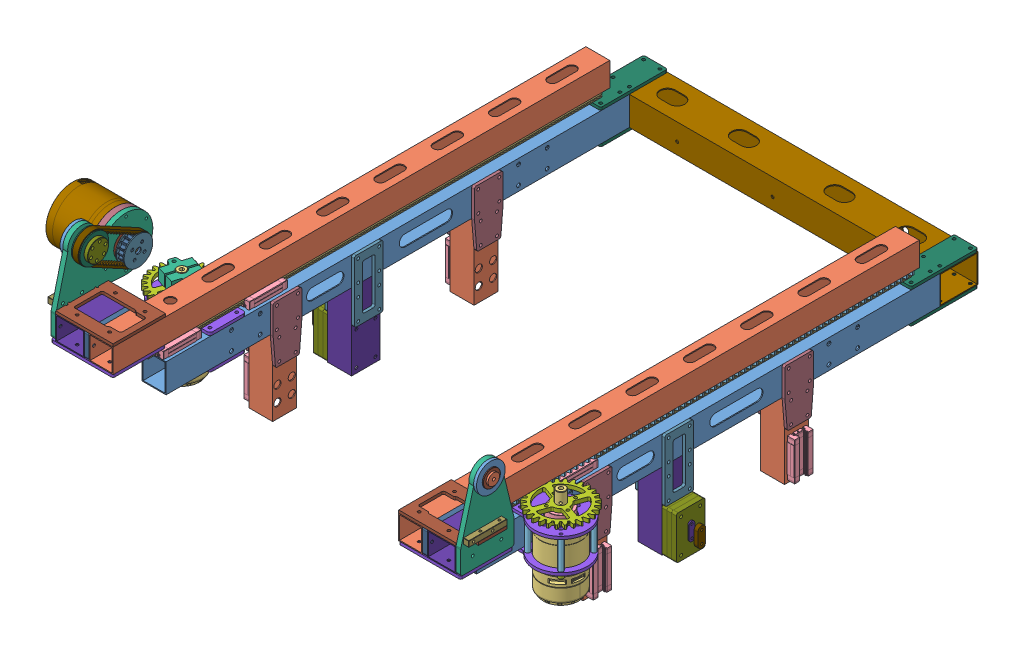
SolidWorks assembly 前探2.0, configuration 默认. Lengths in mm.
Overall size (521.63 224 581.5).
126 component instances, 37 part files, 323 mates.
Components (placement in the parent):
- 30x25x1铝方管-2: 30x25x1铝方管 [前探底管] at (162.5 0 0) size (25 30 485)
- 25x25x1铝方管-1: 25x25x1铝方管 [前探长管镜像] at (-162.5 43.5 38) size (25 25 520)
- 25x25x1铝方管-2: 25x25x1铝方管 [前探长管] at (162.5 43.5 39) size (25 25 520)
- RoboMaster M3508直流无刷减速电机-1: RoboMaster M3508直流无刷减速电机 [默认] at (-216.3113 -71.441 182.0369) x (0.14601 0 0.989283) z (0 1 0) size (42 42.01 98.4)
- 推力球轴承-1: 推力球轴承 [51100 10*24*9] at (-198.5 17 177.6) x (-0.941237 0 -0.337746) z (0.337746 0 -0.941237) size (24 9 24)
- 304不锈钢接线柱-1: 304不锈钢接线柱 [M3*30-5] at (-215.8241 0 160.2759) x (0.012605 0 0.999921) z (0 1 0) size (5 5 30)
- 304不锈钢接线柱-3: 304不锈钢接线柱 [M3*30-5] at (-215.8241 0 194.9241) x (-0.333238 0 0.942843) z (0 1 0) size (5 5 30)
- 304不锈钢接线柱-4: 304不锈钢接线柱 [M3*30-5] at (-181.1759 0 160.2759) x (-0.657276 0 0.75365) z (0 1 0) size (5 5 30)
- RoboMaster M3508直流无刷减速电机-2: RoboMaster M3508直流无刷减速电机 [默认] at (206.3813 -71.441 194.1776) x (0.940674 0 -0.339312) z (0 1 0) size (42 42.01 98.4)
- 推力球轴承-2: 推力球轴承 [51100 10*24*9] at (198.5 17 177.6) x (0.998455 0 0.055559) z (-0.055559 0 0.998455) size (24 9 24)
- 304不锈钢接线柱-5: 304不锈钢接线柱 [M3*30-5] at (215.8241 0 160.2759) x (-0.333238 0 0.942843) z (0 1 0) size (5 5 30)
- 304不锈钢接线柱-6: 304不锈钢接线柱 [M3*30-5] at (215.8241 0 194.9241) x (-0.485899 0 0.874015) z (0 1 0) size (5 5 30)
- 304不锈钢接线柱-7: 304不锈钢接线柱 [M3*30-5] at (181.1759 0 194.9241) x (-0.280607 0 0.959823) z (0 1 0) size (5 5 30)
- 304不锈钢接线柱-8: 304不锈钢接线柱 [M3*30-5] at (181.1759 0 160.2759) x (-0.117969 0 0.993017) z (0 1 0) size (5 5 30)
- 横移连接板-1: 横移连接板 [电机安装板] at (-210 43.5 263) x (0 0 1) z (-1 0 0) size (101.67 92 5)
- 12.9级圆柱头螺钉-2: 12.9级圆柱头螺钉 [M3*8] at (-215.8241 -21 194.9241) x (-0.034714 0 -0.999397) z (0 -1 0) size (5.68 5.68 11)
- 12.9级圆柱头螺钉-3: 12.9级圆柱头螺钉 [M3*8] at (-215.8241 -21 160.2759) x (-0.784933 0 -0.61958) z (0 -1 0) size (5.68 5.68 11)
- 12.9级圆柱头螺钉-4: 12.9级圆柱头螺钉 [M3*8] at (-181.1759 -21 160.2759) x (0.893078 0 -0.449902) z (0 -1 0) size (5.68 5.68 11)
- 12.9级圆柱头螺钉-5: 12.9级圆柱头螺钉 [M3*8] at (181.1759 -21 160.2759) x (0.99769 0 0.06793) z (0 -1 0) size (5.68 5.68 11)
- 12.9级圆柱头螺钉-6: 12.9级圆柱头螺钉 [M3*8] at (215.8241 -21 160.2759) x (0.98152 0 0.19136) z (0 -1 0) size (5.68 5.68 11)
- 12.9级圆柱头螺钉-7: 12.9级圆柱头螺钉 [M3*8] at (215.8241 -21 194.9241) x (0.999534 0 -0.03052) z (0 -1 0) size (5.68 5.68 11)
- 12.9级圆柱头螺钉-8: 12.9级圆柱头螺钉 [M3*8] at (181.1759 -21 194.9241) x (0.99867 0 -0.051563) z (0 -1 0) size (5.68 5.68 11)
- 12.9级圆柱头螺钉-9: 12.9级圆柱头螺钉 [M3*5] at (155 11 230.55) x (0.994595 0 0.103835) z (0 -1 0) size (5.68 5.68 8)
- 12.9级圆柱头螺钉-10: 12.9级圆柱头螺钉 [M3*5] at (170 11 230.55) x (0.998824 0 -0.048475) z (0 -1 0) size (5.68 5.68 8)
- 12.9级圆柱头螺钉-11: 12.9级圆柱头螺钉 [M3*5] at (170 11 214.55) x (0.998723 0 -0.050526) z (0 -1 0) size (5.68 5.68 8)
- 12.9级圆柱头螺钉-12: 12.9级圆柱头螺钉 [M3*5] at (155 11 214.55) x (0.998723 0 -0.050526) z (0 -1 0) size (5.68 5.68 8)
- 12.9级圆柱头螺钉-13: 12.9级圆柱头螺钉 [M3*5] at (170 11 140.65) x (-0.565957 0 0.824435) z (0 -1 0) size (5.68 5.68 8)
- 12.9级圆柱头螺钉-16: 12.9级圆柱头螺钉 [M3*5] at (155 11 140.65) x (0.977106 0 0.212755) z (0 -1 0) size (5.68 5.68 8)
- 12.9级圆柱头螺钉-17: 12.9级圆柱头螺钉 [M3*5] at (170 11 124.65) x (-0.206211 0 0.978508) z (0 -1 0) size (5.68 5.68 8)
- 12.9级圆柱头螺钉-18: 12.9级圆柱头螺钉 [M3*5] at (155 11 124.65) x (0.595095 0 -0.803655) z (0 -1 0) size (5.68 5.68 8)
- 12.9级圆柱头螺钉-19: 12.9级圆柱头螺钉 [M3*5] at (-155 11.0016 230.55) x (0.978167 0 0.207821) z (0 -1 0) size (5.68 5.68 8)
- 12.9级圆柱头螺钉-20: 12.9级圆柱头螺钉 [M3*5] at (-170 11 230.55) x (0.999805 0 0.019757) z (0 -1 0) size (5.68 5.68 8)
- 12.9级圆柱头螺钉-21: 12.9级圆柱头螺钉 [M3*5] at (-155 11.0163 214.55) x (0.980556 0 -0.196239) z (0 -1 0) size (5.68 5.68 8)
- 12.9级圆柱头螺钉-22: 12.9级圆柱头螺钉 [M3*5] at (-170 11 214.55) x (0.907226 0 -0.420643) z (0 -1 0) size (5.68 5.68 8)
- 12.9级圆柱头螺钉-23: 12.9级圆柱头螺钉 [M3*5] at (-155 11 140.65) x (0.937372 0 -0.348331) z (0 -1 0) size (5.68 5.68 8)
- 12.9级圆柱头螺钉-24: 12.9级圆柱头螺钉 [M3*5] at (-170 11 140.65) x (-0.229443 0 -0.973322) z (0 -1 0) size (5.68 5.68 8)
- 12.9级圆柱头螺钉-25: 12.9级圆柱头螺钉 [M3*5] at (-155 11 124.65) x (0.655383 0 -0.755297) z (0 -1 0) size (5.68 5.68 8)
- 12.9级圆柱头螺钉-26: 12.9级圆柱头螺钉 [M3*5] at (-170 11 124.65) x (-0.78488 0 -0.619648) z (0 -1 0) size (5.68 5.68 8)
- 横移连接板-2: 横移连接板 [转轴转点] at (215 43.5 263) x (0 0 1) z (-1 0 0) size (56 92 5)
- 支撑连接板-1: 支撑连接板 [右] at (182.5 28 271.5) x (1 0 0) z (0 1 0) size (65 55 3.23)
- 支撑连接板-2: 支撑连接板 [左] at (-182.5 28 270.5) x (1 0 0) z (0 1 0) size (341.52 580.5 35.52)
- 4310 减速电机 3D 20221104_defeature-1: 4310 减速电机 3D 20221104_defeature [默认] at (-259 83 224.3345) x (0 -0.927289 0.374346) z (0 0.374346 0.927289) size (56 46 56)
- 小带轮-1: 小带轮 [主动轮] at (-205.1 83 224.3345) x (1 0 0) z (0 -0.853122 0.521711) size (7 27.19 27.51)
- 法兰轴承-1: 法兰轴承 [17*26*5-1.1] at (-216.1 83 224.3345) x (0 -0.997676 0.068144) z (0 0.068144 0.997676) size (28 5 28)
- 4310传动法兰-1: 4310传动法兰 [默认] at (-220 83 224.3345) x (0 0.302939 -0.95301) z (1 0 0) size (33 33 19.9)
- 小带轮-2: 小带轮 [从动轮] at (-198.1 108 270.5) x (-1 0 0) z (0 -0.949657 -0.313291) size (7 27.19 27.51)
- 4310安装垫块-1: 4310安装垫块 [默认] at (-215 83 224.3345) x (0 0.536766 0.843731) z (-1 0 0) size (56 56 6)
- 同步带轮挡板-1: 同步带轮挡板 [默认] at (-206.1 83 224.3345) x (0 -0.521711 -0.853122) z (1 0 0) size (30 30 1)
- 同步带轮挡板-2: 同步带轮挡板 [默认] at (-197.1 83 224.3345) x (0 0.521711 0.853122) z (-1 0 0) size (30 30 1)
- 同步带轮挡板1-1: 同步带轮挡板1 [默认] at (-197.1 108 270.5) x (0 0.949657 0.313291) z (-1 0 0) size (30 30 1)
- 同步带轮挡板1-2: 同步带轮挡板1 [默认] at (-206.1 108 270.5) x (0 -0.203511 -0.979073) z (1 0 0) size (30 30 1)
- 横移转点法兰-1: 横移转点法兰 [默认] at (-193 108 270.5) x (0 0.949657 0.313291) z (-1 0 0) size (22 22 26.1)
- 25x30x1铝方管-1: 25x30x1铝方管 [前探管] at (-195 43.5 270.5) size (30 25 55)
- 25x30x1铝方管-2: 25x30x1铝方管 [前探管] at (195 43.5 271.5) size (30 25 55)
- 法兰轴承-2: 法兰轴承 [8*16*5-1.1] at (-208.9 108 270.5) x (0 -0.454379 0.890809) z (0 -0.890809 -0.454379) size (18 5 18)
- 法兰轴承-3: 法兰轴承 [8*16*5-1.1] at (208.9 108 270.5) x (0 -0.670714 0.741716) z (0 0.741716 0.670714) size (18 5 18)
- 同步带1-1: 同步带1 [默认] at (-201.6 108 270.5) x (1 0 0) z (0 0.47619 0.879342) size (6 30.99 83.49)
- 法兰轴承-4: 法兰轴承 [8*16*5-1.1] at (219.1 108 270.5) x (0 -0.846571 -0.532276) z (0 0.532276 -0.846571) size (18 5 18)
- 横移转点垫板-1: 横移转点垫板 [默认] at (215 108 270.5) x (0 -0.116472 -0.993194) z (1 0 0) size (30 30 3)
- 横移转点垫板-2: 横移转点垫板 [默认] at (-218 108 270.5) x (0 0.20708 -0.978324) z (1 0 0) size (30 30 3)
- 法兰轴承-5: 法兰轴承 [8*16*5-1.1] at (-219.1 108 270.5) x (0 -0.931071 0.364837) z (0 0.364837 0.931071) size (18 5 18)
- 转点垫片-1: 转点垫片 [默认] at (-219.1 108 270.5) x (0 0.356837 0.934167) z (-1 0 0) size (12 12 2)
- 转点垫片-2: 转点垫片 [默认] at (221.1 108 270.5) x (0 0.710644 0.703552) z (-1 0 0) size (12 12 2)
- 上银直线导轨线性滑轨MGN-C-O╱MGN-H-O[MGN9H2R475ZACI＋-O]_2-1: 上银直线导轨线性滑轨MGN-C-O╱MGN-H-O[MGN9H2R475ZACI＋-O]_2 [MGN9H-O] at (-162.5 22.8 15.5) x (-1 0 0) z (0 0 1) size (9 6.5 475)
- 上银直线导轨线性滑轨MGN-C-O╱MGN-H-O[MGN9H2R475ZACI＋-O]_1-1: 上银直线导轨线性滑轨MGN-C-O╱MGN-H-O[MGN9H2R475ZACI＋-O]_1 [MGN9H-O] at (-162.5 22.8 222.55) x (-1 0 0) z (0 0 1) size (20 7.8 39.98)
- 上银直线导轨线性滑轨MGN-C-O╱MGN-H-O[MGN9H2R475ZACI＋-O]_1-2: 上银直线导轨线性滑轨MGN-C-O╱MGN-H-O[MGN9H2R475ZACI＋-O]_1 [MGN9H-O] at (-162.5 22.8 132.65) x (-1 0 0) z (0 0 1) size (20 7.8 39.98)
- 30x25x1铝方管-6: 30x25x1铝方管 [前探底管] at (-162.5 0 0) size (25 30 485)
- 上银直线导轨线性滑轨MGN-C-O╱MGN-H-O[MGN9H2R475ZACI＋-O]_2-2: 上银直线导轨线性滑轨MGN-C-O╱MGN-H-O[MGN9H2R475ZACI＋-O]_2 [MGN9H-O] at (162.5 22.8 16.5) x (-1 0 0) z (0 0 1) size (9 6.5 475)
- 上银直线导轨线性滑轨MGN-C-O╱MGN-H-O[MGN9H2R475ZACI＋-O]_1-3: 上银直线导轨线性滑轨MGN-C-O╱MGN-H-O[MGN9H2R475ZACI＋-O]_1 [MGN9H-O] at (162.5 22.8 222.55) x (-1 0 0) z (0 0 1) size (20 7.8 39.98)
- 上银直线导轨线性滑轨MGN-C-O╱MGN-H-O[MGN9H2R475ZACI＋-O]_1-4: 上银直线导轨线性滑轨MGN-C-O╱MGN-H-O[MGN9H2R475ZACI＋-O]_1 [MGN9H-O] at (162.5 22.8 132.65) x (-1 0 0) z (0 0 1) size (20 7.8 39.98)
- 齿条2X76-1: 齿条2X76 [默认] at (168 31 244) x (0 0 -1) z (0 -1 0) size (465 14.5 6)
- 齿条2X76-3: 齿条2X76 [默认] at (-168 25 243) x (0 0 -1) z (0 1 0) size (465 14.5 6)
- 2孔夹紧联轴器-1: 2孔夹紧联轴器 [默认] at (-198.5 30 177.6) x (-0.289177 0 0.957276) z (0 1 0) size (28 32 12)
- 3508前探电机安装板-3: 3508前探电机安装板 [默认] at (-225 19 185.3862) x (0 0 1) z (0 -1 0) size (80 120 0)
- 圆柱齿轮28×2-1: 圆柱齿轮28×2 [默认] at (-198.5 30 177.6) x (0.942893 0 0.333096) z (0 -1 0) size (59.77 59.77 4)
- 前探3508安装板-1: 前探3508安装板 [3508安装板] at (-198.5 16.5 177.6) x (0 0 -1) z (0 1 0) size (55 76 3)
- 2孔夹紧联轴器-2: 2孔夹紧联轴器 [默认] at (198.5 30 177.6) x (-0.289177 0 0.957276) z (0 1 0) size (28 32 12) (hidden)
- 圆柱齿轮28×2-2: 圆柱齿轮28×2 [默认] at (198.5 30 177.6) x (0.942893 0 0.333096) z (0 -1 0) size (59.77 59.77 4)
- 前探3508安装板-2: 前探3508安装板 [3508安装板] at (198.5 16.5 177.6) x (0 0 -1) z (0 -1 0) size (55 76 3)
- 40x30x1铝方管-1: 40x30x1铝方管 [默认] at (0 0 -262.5) x (0 0 1) z (-1 0 0) size (40 30 350)
- 前探3508安装板-3: 前探3508安装板 [下端固定板] at (-198.5 -16.5 177.6) x (0 0 -1) z (0 1 0) size (55 76 3)
- 304不锈钢接线柱-9: 304不锈钢接线柱 [M3*30-5] at (-181.1759 0 194.9241) x (-0.000437 0 1) z (0 1 0) size (5 5 30)
- 12.9级圆柱头螺钉-27: 12.9级圆柱头螺钉 [M3*8] at (-181.1759 -21 194.9241) x (-0.034714 0 -0.999397) z (0 -1 0) size (5.68 5.68 11)
- 前探3508安装板-4: 前探3508安装板 [下端固定板] at (198.5 -16.5 177.6) x (0 0 -1) z (0 -1 0) size (55 76 3)
- 25x25x1铝方管-3: 25x25x1铝方管 [抬升滑块安装管] at (162.5 -55 118.4) x (1 0 0) z (0 -1 0) size (25 25 80)
- 25x25x1铝方管-4: 25x25x1铝方管 [抬升滑块安装管] at (162.5 -55 -92.4) x (1 0 0) z (0 -1 0) size (25 25 80)
- 上银直线导轨线性滑轨MGN-C-O╱MGN-H-O[MGN9H2R475ZACI＋-O]_1-5: 上银直线导轨线性滑轨MGN-C-O╱MGN-H-O[MGN9H2R475ZACI＋-O]_1 [MGN9H-O] at (182.8 -72.05 118.4) x (0 0 -1) z (0 1 0) size (20 7.8 39.98)
- 上银直线导轨线性滑轨MGN-C-O╱MGN-H-O[MGN9H2R475ZACI＋-O]_1-6: 上银直线导轨线性滑轨MGN-C-O╱MGN-H-O[MGN9H2R475ZACI＋-O]_1 [MGN9H-O] at (182.8 -72.05 -92.4) x (0 0 -1) z (0 1 0) size (20 7.8 39.98)
- 25x25x1铝方管-5: 25x25x1铝方管 [抬升滑块安装管] at (-162.5 -55 118.4) x (-1 0 0) z (0 -1 0) size (25 25 80)
- 25x25x1铝方管-6: 25x25x1铝方管 [抬升滑块安装管] at (-162.5 -55 -92.4) x (-1 0 0) z (0 -1 0) size (25 25 80)
- 上银直线导轨线性滑轨MGN-C-O╱MGN-H-O[MGN9H2R475ZACI＋-O]_1-7: 上银直线导轨线性滑轨MGN-C-O╱MGN-H-O[MGN9H2R475ZACI＋-O]_1 [MGN9H-O] at (-182.8 -72.05 -92.4) x (0 0 -1) z (0 -1 0) size (20 7.8 39.98)
- 上银直线导轨线性滑轨MGN-C-O╱MGN-H-O[MGN9H2R475ZACI＋-O]_1-8: 上银直线导轨线性滑轨MGN-C-O╱MGN-H-O[MGN9H2R475ZACI＋-O]_1 [MGN9H-O] at (-182.8 -72.05 118.4) x (0 0 -1) z (0 -1 0) size (20 7.8 39.98)
- 前探垫块-1: 前探垫块 [默认] at (-180 43.5 270.5) x (0 0 -1) z (1 0 0) size (55 25 5)
- 前探垫块-2: 前探垫块 [默认] at (175 43.5 271.5) x (0 0 -1) z (1 0 0) size (55 25 5)
- 前探加固板-1: 前探加固板 [默认] at (-180 59 270.5) x (0 0 1) z (0 -1 0) size (55 71 3)
- 四孔直角转接件-1: 四孔直角转接件 [上交角件] at (-218 62 275.5) x (0 1 0) z (0 0 1) size (6 6 40)
- 前探加固板-2: 前探加固板 [默认] at (180 56 271.5) x (0 0 1) z (0 1 0) size (55 71 3)
- 四孔直角转接件-2: 四孔直角转接件 [上交角件] at (218 62 276.5) x (0 1 0) z (0 0 1) size (6 6 40)
- 25x30x1铝方管-3: 25x30x1铝方管 [抬升管] at (-162.5 -55 33.295) x (0 0 1) z (0 1 0) size (30 25 80)
- 25x30x1铝方管-4: 25x30x1铝方管 [抬升管] at (162.5 -55 33.295) x (0 0 -1) z (0 1 0) size (30 25 80)
- 抬升连接板1-1: 抬升连接板1 [默认] at (-176.5 0 -92.4) x (0 0 1) z (-1 0 0) size (30 60 3)
- 抬升连接板1-2: 抬升连接板1 [默认] at (-176.5 0 118.4) x (0 0 -1) z (1 0 0) size (30 60 3)
- 抬升连接板1-3: 抬升连接板1 [默认] at (-148.5 0 -92.4) x (0 0 1) z (-1 0 0) size (30 60 3)
- 抬升连接板1-4: 抬升连接板1 [默认] at (-148.5 0 118.4) x (0 0 -1) z (1 0 0) size (30 60 3)
- 抬升连接板2-1: 抬升连接板2 [默认] at (-175 -17.5 33.295) x (0 0 1) z (-1 0 0) size (30 65 3)
- 抬升连接板2-2: 抬升连接板2 [默认] at (-147 -17.5 33.295) x (0 0 1) z (-1 0 0) size (30 65 3)
- 抬升连接板1-5: 抬升连接板1 [默认] at (176.5 0 118.4) x (0 0 -1) z (1 0 0) size (30 60 3)
- 抬升连接板1-6: 抬升连接板1 [默认] at (148.5 0 118.4) x (0 0 -1) z (1 0 0) size (30 60 3)
- 抬升连接板1-7: 抬升连接板1 [默认] at (176.5 0 -92.4) x (0 0 -1) z (1 0 0) size (30 60 3)
- 抬升连接板1-8: 抬升连接板1 [默认] at (148.5 0 -92.4) x (0 0 -1) z (1 0 0) size (30 60 3)
- 抬升连接板2-3: 抬升连接板2 [默认] at (178 -17.5 33.295) x (0 0 1) z (-1 0 0) size (30 65 3)
- 抬升连接板2-4: 抬升连接板2 [默认] at (150 -17.5 33.295) x (0 0 1) z (-1 0 0) size (30 65 3)
- 前探连接板-1: 前探连接板 [默认] at (-162.5 15 -247.5) x (0 0 -1) z (0 1 0) size (70 25 3)
- 前探连接板-2: 前探连接板 [默认] at (162.5 15 -247.5) x (0 0 -1) z (0 1 0) size (70 25 3)
- 前探连接板-3: 前探连接板 [默认] at (162.5 -18 -247.5) x (0 0 -1) z (0 1 0) size (70 25 3)
- 前探连接板-4: 前探连接板 [默认] at (-162.5 -18 -247.5) x (0 0 -1) z (0 1 0) size (70 25 3)
- 抬升链条连接-1: 抬升链条连接 [底层] at (-175 -72.5 33.295) x (0 0 1) z (-1 0 0) size (30 45 5)
- 抬升链条连接-2: 抬升链条连接 [二层] at (-180 -72.5 33.295) x (0 0 1) z (-1 0 0) size (30 45 5)
- 抬升链条连接-5: 抬升链条连接 [连接一层] at (-185 -72.5 33.295) x (0 0 1) z (-1 0 0) size (30 45 5)
- 链条连接垫块-1: 链条连接垫块 [默认] at (-190 -72.5 33.295) x (0 0 1) z (-1 0 0) size (6 18.7 1.31)
- 链条连接-1: 链条连接 [默认] at (-197.69 -72.5 33.295) x (0 0 1) z (-1 0 0) size (8 20.7 4)
- 抬升链条连接-6: 抬升链条连接 [底层] at (180 -72.5 33.295) x (0 0 1) z (-1 0 0) size (30 45 5)
- 抬升链条连接-8: 抬升链条连接 [底层] at (185 -72.5 33.295) x (0 0 1) z (-1 0 0) size (30 45 5)
- 抬升链条连接-9: 抬升链条连接 [连接一层] at (190 -72.5 33.295) x (0 0 1) z (-1 0 0) size (30 45 5)
- 链条连接垫块-2: 链条连接垫块 [默认] at (191.31 -72.5 33.295) x (0 0 1) z (-1 0 0) size (6 18.7 1.31)
- 链条连接-2: 链条连接 [默认] at (201.69 -72.5 33.295) x (0 0 1) z (-1 0 0) size (8 20.7 4)
Mates (geometry in assembly coordinates):
- 重合3: coincident aligned: plane of 30x25x1铝方管-2 through (162.5 0 0) normal (0 0 1)
- 重合4: coincident aligned: plane of 30x25x1铝方管-2 through (162.5 0 0) normal (0 1 0)
- 同心2: concentric anti-aligned: cylinder of RoboMaster M3508直流无刷减速电机-1 through (-198.5 42.3 177.6) axis (0 1 0) radius 5; cylinder of 推力球轴承-1 through (-198.5 26 177.6) axis (0 -1 0) radius 12
- 重合23: coincident anti-aligned: plane of RoboMaster M3508直流无刷减速电机-1 through (-209.1562 17 174.8713) normal (0 1 0); plane of 推力球轴承-1 through (-198.5 17 177.6) normal (0 -1 0)
- 同心19: concentric anti-aligned: cylinder of RoboMaster M3508直流无刷减速电机-2 through (198.5 42.3 177.6) axis (0 1 0) radius 5; cylinder of 推力球轴承-2 through (198.5 26 177.6) axis (0 -1 0) radius 5
- 重合44: coincident anti-aligned: plane of RoboMaster M3508直流无刷减速电机-2 through (197.9389 17 188.5857) normal (0 1 0); plane of 推力球轴承-2 through (198.5 17 177.6) normal (0 -1 0)
- 重合54: coincident aligned: plane of 25x25x1铝方管-1 through (-175 31 298) normal (0 -1 0); plane of 横移连接板-1 through (-215 31 243) normal (0 -1 0)
- 重合68: coincident anti-aligned: plane of 30x25x1铝方管-2 through (151 14 242.5) normal (0 -1 0); plane of 12.9级圆柱头螺钉-9 through (154.7051 14 233.3746) normal (0 1 0)
- 重合691: coincident anti-aligned: plane of 30x25x1铝方管-2 through (151 14 242.5) normal (0 -1 0); plane of 12.9级圆柱头螺钉-10 through (170.1377 14 233.3867) normal (0 1 0)
- 重合701: coincident anti-aligned: plane of 30x25x1铝方管-2 through (151 14 242.5) normal (0 -1 0); plane of 12.9级圆柱头螺钉-11 through (170.1435 14 217.3864) normal (0 1 0)
- 重合711: coincident anti-aligned: plane of 30x25x1铝方管-2 through (151 14 242.5) normal (0 -1 0); plane of 12.9级圆柱头螺钉-12 through (155.1435 14 217.3864) normal (0 1 0)
- 重合72: coincident anti-aligned: plane of 30x25x1铝方管-2 through (151 14 242.5) normal (0 -1 0); plane of 12.9级圆柱头螺钉-13 through (167.6586 14 139.0427) normal (0 1 0)
- 重合761: coincident anti-aligned: plane of 30x25x1铝方管-2 through (151 14 242.5) normal (0 -1 0); plane of 12.9级圆柱头螺钉-16 through (154.3958 14 143.425) normal (0 1 0)
- 重合77: coincident anti-aligned: plane of 30x25x1铝方管-2 through (151 14 242.5) normal (0 -1 0); plane of 12.9级圆柱头螺钉-17 through (167.221 14 124.0644) normal (0 1 0)
- 重合78: coincident anti-aligned: plane of 30x25x1铝方管-2 through (151 14 242.5) normal (0 -1 0); plane of 12.9级圆柱头螺钉-18 through (157.2824 14 126.3401) normal (0 1 0)
- 平行8: parallel aligned: plane of 25x25x1铝方管-2 through (150 31 299) normal (0 -1 0); plane of 横移连接板-2 through (210 31 243) normal (0 -1 0)
- 同心427: concentric aligned: cylinder of 横移连接板-1 through (-224 108 270.5) axis (1 0 0) radius 8; cylinder of 横移连接板-2 through (201 108 270.5) axis (1 0 0) radius 8
- 重合786: coincident anti-aligned: plane of 25x25x1铝方管-2 through (150 31 299) normal (0 -1 0); plane of 支撑连接板-1 through (182.5 31 271.5) normal (0 1 0)
- 重合787: coincident aligned: plane of 25x25x1铝方管-2 through (150 31 299) normal (-1 0 0); plane of 支撑连接板-1 through (150 31 299) normal (-1 0 0)
- 重合788: coincident aligned: plane of 25x25x1铝方管-2 through (162.5 43.5 299) normal (0 0 1); plane of 支撑连接板-1 through (150 31 299) normal (0 0 1)
- 重合789: coincident anti-aligned: plane of 25x25x1铝方管-1 through (-175 31 298) normal (0 -1 0); plane of 支撑连接板-2 through (-182.5 31 270.5) normal (0 1 0)
- 重合790: coincident aligned: plane of 25x25x1铝方管-1 through (-150 31 298) normal (1 0 0); plane of 支撑连接板-2 through (-150 31 298) normal (1 0 0)
- 重合791: coincident aligned: plane of 25x25x1铝方管-1 through (-162.5 43.5 298) normal (0 0 1); plane of 支撑连接板-2 through (-215 31 298) normal (0 0 1)
- 重合792: coincident aligned: plane of 25x25x1铝方管-1 through (-162.5 43.5 298) normal (0 0 1); plane of 横移连接板-1 through (-301.6256 31 298) normal (0 0 1)
- 同心428: concentric anti-aligned: cylinder of 横移连接板-1 through (-220 83 224.3345) axis (1 0 0) radius 13; cylinder of 法兰轴承-1 through (-211.1 83 224.3345) axis (-1 0 0) radius 13
- 重合793: coincident anti-aligned: plane of 横移连接板-1 through (-215 43.5 263) normal (-1 0 0); plane of 法兰轴承-1 through (-215 83 224.3345) normal (1 0 0)
- 同心429: concentric aligned: cylinder of 4310 减速电机 3D 20221104_defeature-1 through (-259 83 224.3345) axis (-1 0 0) radius 28; cylinder of 法兰轴承-1 through (-211.1 83 224.3345) axis (-1 0 0) radius 8.5
- 距离15: distance = 6 mm anti-aligned: plane of 4310 减速电机 3D 20221104_defeature-1 through (-221 63.0633 232.383) normal (1 0 0); plane of 横移连接板-1 through (-215 43.5 263) normal (-1 0 0)
- 同心430: concentric aligned: cylinder of 法兰轴承-1 through (-211.1 83 224.3345) axis (-1 0 0) radius 8.5; cylinder of 4310传动法兰-1 through (-206.1 83 224.3345) axis (-1 0 0) radius 8.5
- 重合794: coincident anti-aligned: plane of 4310 减速电机 3D 20221104_defeature-1 through (-220 84.7781 228.7392) normal (1 0 0); plane of 4310传动法兰-1 through (-220 83 224.3345) normal (-1 0 0)
- 同心431: concentric anti-aligned: cylinder of 小带轮-1 through (-208.1 83 224.3345) axis (1 0 0) radius 3; cylinder of 4310传动法兰-1 through (-206.1 83 224.3345) axis (-1 0 0) radius 8.5
- 同心432: concentric anti-aligned: cylinder of 横移连接板-1 through (-224 108 270.5) axis (1 0 0) radius 8; cylinder of 小带轮-2 through (-195.1 108 270.5) axis (-1 0 0) radius 5
- 同心433: concentric aligned: cylinder of 4310 减速电机 3D 20221104_defeature-1 through (-221 83 224.3345) axis (1 0 0) radius 28; cylinder of 4310安装垫块-1 through (-221 83 224.3345) axis (1 0 0) radius 28
- 重合796: coincident anti-aligned: plane of 横移连接板-1 through (-215 43.5 263) normal (-1 0 0); plane of 4310安装垫块-1 through (-215 83 224.3345) normal (1 0 0)
- 同心434: concentric anti-aligned: cylinder of 4310传动法兰-1 through (-200.1 83 224.3345) axis (-1 0 0) radius 3; cylinder of 同步带轮挡板-1 through (-206.1 83 224.3345) axis (1 0 0) radius 3
- 重合797: coincident anti-aligned: plane of 4310传动法兰-1 through (-206.1 83 224.3345) normal (1 0 0); plane of 同步带轮挡板-1 through (-206.1 83 224.3345) normal (-1 0 0)
- 重合798: coincident anti-aligned: plane of 小带轮-1 through (-205.1 84.435 226.6811) normal (-1 0 0); plane of 同步带轮挡板-1 through (-205.1 83 224.3345) normal (1 0 0)
- 同心435: concentric anti-aligned: cylinder of 小带轮-1 through (-244.1 86.9128 230.733) axis (1 0 0) radius 1.525; cylinder of 同步带轮挡板-1 through (-205.1 86.9128 230.733) axis (-1 0 0) radius 1.525
- 重合800: coincident anti-aligned: plane of 小带轮-1 through (-198.1 84.435 226.6811) normal (1 0 0); plane of 同步带轮挡板-2 through (-198.1 83 224.3345) normal (-1 0 0)
- 同心436: concentric anti-aligned: cylinder of 小带轮-1 through (-208.1 83 224.3345) axis (1 0 0) radius 3; cylinder of 同步带轮挡板-2 through (-197.1 83 224.3345) axis (-1 0 0) radius 3
- 同心437: concentric aligned: cylinder of 小带轮-1 through (-244.1 86.9128 230.733) axis (1 0 0) radius 1.525; cylinder of 同步带轮挡板-2 through (-198.1 86.9128 230.733) axis (1 0 0) radius 1.525
- 重合801: coincident aligned: plane of 小带轮-1 through (-198.1 84.435 226.6811) normal (1 0 0); plane of 小带轮-2 through (-198.1 108.8617 267.8879) normal (1 0 0)
- 重合802: coincident anti-aligned: plane of 小带轮-2 through (-198.1 108.8617 267.8879) normal (1 0 0); plane of 同步带轮挡板1-1 through (-198.1 108 270.5) normal (-1 0 0)
- 同心438: concentric anti-aligned: cylinder of 小带轮-2 through (-173.1 115.8326 268.8719) axis (-1 0 0) radius 1.5; cylinder of 同步带轮挡板1-1 through (-198.1 115.8326 268.8719) axis (1 0 0) radius 1.5
- 同心439: concentric anti-aligned: cylinder of 小带轮-2 through (-195.1 108 270.5) axis (-1 0 0) radius 5; cylinder of 同步带轮挡板1-1 through (-198.1 108 270.5) axis (1 0 0) radius 5
- 重合8031: coincident anti-aligned: plane of 小带轮-2 through (-205.1 108.8617 267.8879) normal (-1 0 0); plane of 同步带轮挡板1-2 through (-205.1 108 270.5) normal (1 0 0)
- 同心440: concentric aligned: cylinder of 小带轮-2 through (-195.1 108 270.5) axis (-1 0 0) radius 5; cylinder of 同步带轮挡板1-2 through (-205.1 108 270.5) axis (-1 0 0) radius 5
- 同心441: concentric anti-aligned: cylinder of 同步带轮挡板1-1 through (-198.1 113.3263 276.4692) axis (1 0 0) radius 1.5; cylinder of 同步带轮挡板1-2 through (-205.1 113.3263 276.4692) axis (-1 0 0) radius 1.5
- 同心442: concentric anti-aligned: cylinder of 小带轮-2 through (-195.1 108 270.5) axis (-1 0 0) radius 5; cylinder of 横移转点法兰-1 through (-219.1 108 270.5) axis (1 0 0) radius 5
- 重合804: coincident anti-aligned: plane of 同步带轮挡板1-1 through (-197.1 108 270.5) normal (1 0 0); plane of 横移转点法兰-1 through (-197.1 108 270.5) normal (-1 0 0)
- 同心443: concentric aligned: cylinder of 同步带轮挡板1-1 through (-198.1 113.3263 276.4692) axis (1 0 0) radius 1.5; cylinder of 横移转点法兰-1 through (-197.1 113.3263 276.4692) axis (1 0 0) radius 1.5
- 重合806: coincident aligned: plane of 25x25x1铝方管-1 through (-162.5 43.5 298) normal (0 0 1); plane of 25x30x1铝方管-1 through (-195 43.5 298) normal (0 0 1)
- 重合807: coincident anti-aligned: plane of 支撑连接板-2 through (-182.5 31 270.5) normal (0 1 0); plane of 25x30x1铝方管-1 through (-210 31 298) normal (0 -1 0)
- 重合808: coincident anti-aligned: plane of 横移连接板-1 through (-210 43.5 263) normal (1 0 0); plane of 25x30x1铝方管-1 through (-210 31 298) normal (-1 0 0)
- 重合810: coincident aligned: plane of 支撑连接板-1 through (150 31 299) normal (0 0 1); plane of 25x30x1铝方管-2 through (195 43.5 299) normal (0 0 1)
- 重合811: coincident anti-aligned: plane of 支撑连接板-1 through (182.5 31 271.5) normal (0 1 0); plane of 25x30x1铝方管-2 through (180 31 299) normal (0 -1 0)
- 重合812: coincident anti-aligned: plane of 横移连接板-2 through (210 43.5 263) normal (-1 0 0); plane of 25x30x1铝方管-2 through (210 31 299) normal (1 0 0)
- 同心444: concentric aligned: cylinder of 横移连接板-1 through (-224 108 270.5) axis (1 0 0) radius 8; cylinder of 法兰轴承-2 through (-213.9 108 270.5) axis (1 0 0) radius 8
- 重合815: coincident anti-aligned: plane of 横移连接板-1 through (-210 43.5 263) normal (1 0 0); plane of 法兰轴承-2 through (-210 108 270.5) normal (-1 0 0)
- 同心445: concentric anti-aligned: cylinder of 横移连接板-2 through (201 108 270.5) axis (1 0 0) radius 8; cylinder of 法兰轴承-3 through (213.9 108 270.5) axis (-1 0 0) radius 8
- 重合816: coincident anti-aligned: plane of 横移连接板-2 through (210 43.5 263) normal (-1 0 0); plane of 法兰轴承-3 through (210 108 270.5) normal (1 0 0)
- 同心446: concentric aligned: cylinder of 同步带轮挡板-2 through (-198.1 83 224.3345) axis (1 0 0) radius 15; cylinder of 同步带1-1 through (-201.6 83 224.3345) axis (1 0 0) radius 15.493
- 同心447: concentric anti-aligned: cylinder of 同步带轮挡板1-1 through (-198.1 108 270.5) axis (1 0 0) radius 15; cylinder of 同步带1-1 through (-201.6 108 270.5) axis (-1 0 0) radius 15.493
- 宽度13: width anti-aligned: plane of 同步带1-1 through (-204.6 97.7179 276.0681) normal (-1 0 0); plane of 同步带1-1 through (-198.6 94.3764 277.8776) normal (1 0 0); plane of 同步带轮挡板-1 through (-205.1 83 224.3345) normal (1 0 0); plane of 同步带轮挡板-2 through (-198.1 83 224.3345) normal (-1 0 0)
- 同心448: concentric anti-aligned: cylinder of 法兰轴承-3 through (213.9 108 270.5) axis (-1 0 0) radius 4; cylinder of 法兰轴承-4 through (214.1 108 270.5) axis (1 0 0) radius 4
- 距离16: distance = 0.2 mm anti-aligned: plane of 法兰轴承-3 through (213.9 108 270.5) normal (1 0 0); plane of 法兰轴承-4 through (214.1 108 270.5) normal (-1 0 0)
- 同心449: concentric anti-aligned: cylinder of 法兰轴承-4 through (214.1 108 270.5) axis (1 0 0) radius 4; cylinder of 横移转点垫板-1 through (218 108 270.5) axis (-1 0 0) radius 8
- 重合8032: coincident anti-aligned: plane of 横移连接板-2 through (215 43.5 263) normal (1 0 0); plane of 横移转点垫板-1 through (215 108 270.5) normal (-1 0 0)
- 同心450: concentric anti-aligned: cylinder of 横移连接板-1 through (-257.4264 108 270.5) axis (1 0 0) radius 15; cylinder of 横移转点垫板-2 through (-215 108 270.5) axis (-1 0 0) radius 15
- 重合8033: coincident anti-aligned: plane of 横移连接板-1 through (-215 43.5 263) normal (-1 0 0); plane of 横移转点垫板-2 through (-215 108 270.5) normal (1 0 0)
- 同心451: concentric aligned: cylinder of 横移转点垫板-2 through (-215 108 270.5) axis (-1 0 0) radius 8; cylinder of 法兰轴承-5 through (-214.1 108 270.5) axis (-1 0 0) radius 8
- 重合8034: coincident anti-aligned: plane of 横移转点垫板-2 through (-218 108 270.5) normal (-1 0 0); plane of 法兰轴承-5 through (-218 108 270.5) normal (1 0 0)
- 同心452: concentric anti-aligned: cylinder of 横移转点法兰-1 through (-219.1 108 270.5) axis (-1 0 0) radius 1.25; cylinder of 转点垫片-1 through (-221.1 108 270.5) axis (1 0 0) radius 1.55
- 重合8035: coincident anti-aligned: plane of 法兰轴承-5 through (-219.1 108 270.5) normal (-1 0 0); plane of 转点垫片-1 through (-219.1 108 270.5) normal (1 0 0)
- 同心453: concentric anti-aligned: cylinder of 法兰轴承-3 through (213.9 108 270.5) axis (-1 0 0) radius 4; cylinder of 转点垫片-2 through (219.1 108 270.5) axis (1 0 0) radius 1.55
- 重合8036: coincident anti-aligned: plane of 法兰轴承-4 through (219.1 108 270.5) normal (1 0 0); plane of 转点垫片-2 through (219.1 108 270.5) normal (-1 0 0)
- 宽度14: width aligned: plane of 25x25x1铝方管-1 through (-150 31 298) normal (1 0 0); plane of 上银直线导轨线性滑轨MGN-C-O╱MGN-H-O[MGN9H2R475ZACI＋-O]_2-1 through (-175 31 298) normal (-1 0 0); plane of 25x25x1铝方管-1 through (-158 24.6775 253) normal (1 0 0); plane of 上银直线导轨线性滑轨MGN-C-O╱MGN-H-O[MGN9H2R475ZACI＋-O]_2-1 through (-167 24.6775 253) normal (-1 0 0)
- 重合8044: coincident anti-aligned: plane of 上银直线导轨线性滑轨MGN-C-O╱MGN-H-O[MGN9H2R475ZACI＋-O]_2-1 through (-166.6775 18.5 253) normal (0 -1 0); plane of 上银直线导轨线性滑轨MGN-C-O╱MGN-H-O[MGN9H2R475ZACI＋-O]_1-1 through (-166.6775 18.5 203.925) normal (0 1 0)
- 宽度15: width anti-aligned: plane of 上银直线导轨线性滑轨MGN-C-O╱MGN-H-O[MGN9H2R475ZACI＋-O]_1-1 through (-167 24.6775 203.925) normal (1 0 0); plane of 上银直线导轨线性滑轨MGN-C-O╱MGN-H-O[MGN9H2R475ZACI＋-O]_2-1 through (-158 24.6775 203.925) normal (-1 0 0); plane of 上银直线导轨线性滑轨MGN-C-O╱MGN-H-O[MGN9H2R475ZACI＋-O]_1-1 through (-167 24.6775 253) normal (-1 0 0); plane of 上银直线导轨线性滑轨MGN-C-O╱MGN-H-O[MGN9H2R475ZACI＋-O]_2-1 through (-158 24.6775 253) normal (1 0 0)
- 宽度18: width anti-aligned: plane of 上银直线导轨线性滑轨MGN-C-O╱MGN-H-O[MGN9H2R475ZACI＋-O]_1-2 through (-172.5 17 147.3) normal (-1 0 0); plane of 上银直线导轨线性滑轨MGN-C-O╱MGN-H-O[MGN9H2R475ZACI＋-O]_2-1 through (-152.5 17 147.3) normal (1 0 0); plane of 上银直线导轨线性滑轨MGN-C-O╱MGN-H-O[MGN9H2R475ZACI＋-O]_1-2 through (-158 24.6775 253) normal (1 0 0); plane of 上银直线导轨线性滑轨MGN-C-O╱MGN-H-O[MGN9H2R475ZACI＋-O]_2-1 through (-167 24.6775 253) normal (-1 0 0)
- 距离18: distance = 50 mm anti-aligned: plane of 上银直线导轨线性滑轨MGN-C-O╱MGN-H-O[MGN9H2R475ZACI＋-O]_1-2 through (-162.5 32.2555 152.6) normal (0 0 1); plane of 上银直线导轨线性滑轨MGN-C-O╱MGN-H-O[MGN9H2R475ZACI＋-O]_1-1 through (-162.5 32.2555 202.6) normal (0 0 -1)
- 同心459: concentric anti-aligned: cylinder of 12.9级圆柱头螺钉-22 through (-170 19 214.55) axis (0 1 0) radius 1.5; cylinder of 上银直线导轨线性滑轨MGN-C-O╱MGN-H-O[MGN9H2R475ZACI＋-O]_1-1 through (-170 15 214.55) axis (0 -1 0) radius 1.5
- 同心460: concentric anti-aligned: cylinder of 12.9级圆柱头螺钉-25 through (-155 19 124.65) axis (0 1 0) radius 1.5; cylinder of 上银直线导轨线性滑轨MGN-C-O╱MGN-H-O[MGN9H2R475ZACI＋-O]_1-2 through (-155 15 124.65) axis (0 -1 0) radius 1.5
- 同心461: concentric anti-aligned: cylinder of 12.9级圆柱头螺钉-26 through (-170 19 124.65) axis (0 1 0) radius 1.5; cylinder of 上银直线导轨线性滑轨MGN-C-O╱MGN-H-O[MGN9H2R475ZACI＋-O]_1-2 through (-170 15 124.65) axis (0 -1 0) radius 1.5
- 同心462: concentric anti-aligned: cylinder of 12.9级圆柱头螺钉-24 through (-170 19 140.65) axis (0 1 0) radius 1.5; cylinder of 上银直线导轨线性滑轨MGN-C-O╱MGN-H-O[MGN9H2R475ZACI＋-O]_1-2 through (-170 15 140.65) axis (0 -1 0) radius 1.5
- 同心463: concentric anti-aligned: cylinder of 12.9级圆柱头螺钉-23 through (-155 19 140.65) axis (0 1 0) radius 1.5; cylinder of 上银直线导轨线性滑轨MGN-C-O╱MGN-H-O[MGN9H2R475ZACI＋-O]_1-2 through (-155 15 140.65) axis (0 -1 0) radius 1.5
- 同心464: concentric anti-aligned: cylinder of 12.9级圆柱头螺钉-19 through (-155 19.0016 230.55) axis (0 1 0) radius 1.5; cylinder of 上银直线导轨线性滑轨MGN-C-O╱MGN-H-O[MGN9H2R475ZACI＋-O]_1-1 through (-155 15 230.55) axis (0 -1 0) radius 1.5
- 同心465: concentric anti-aligned: cylinder of 12.9级圆柱头螺钉-21 through (-155 19.0163 214.55) axis (0 1 0) radius 1.5; cylinder of 上银直线导轨线性滑轨MGN-C-O╱MGN-H-O[MGN9H2R475ZACI＋-O]_1-1 through (-155 15 214.55) axis (0 -1 0) radius 1.5
- 同心466: concentric anti-aligned: cylinder of 12.9级圆柱头螺钉-20 through (-170 19 230.55) axis (0 1 0) radius 1.5; cylinder of 上银直线导轨线性滑轨MGN-C-O╱MGN-H-O[MGN9H2R475ZACI＋-O]_1-1 through (-170 15 230.55) axis (0 -1 0) radius 1.5
- 同心467: concentric anti-aligned: cylinder of 12.9级圆柱头螺钉-22 through (-170 19 214.55) axis (0 1 0) radius 1.5; cylinder of 上银直线导轨线性滑轨MGN-C-O╱MGN-H-O[MGN9H2R475ZACI＋-O]_1-1 through (-170 15 214.55) axis (0 -1 0) radius 1.5
- 对称1: symmetric aligned: plane of 30x25x1铝方管-2 through (150 -15 242.5) normal (-1 0 0); plane of 30x25x1铝方管-6 through (-150 -15 242.5) normal (1 0 0)
- 重合8050: coincident aligned: plane of 30x25x1铝方管-2 through (150 -15 242.5) normal (0 -1 0); plane of 30x25x1铝方管-6 through (-175 -15 242.5) normal (0 -1 0)
- 重合8051: coincident aligned: plane of 30x25x1铝方管-2 through (162.5 0 0) normal (0 1 0)
- 重合8052: coincident aligned: plane of 30x25x1铝方管-2 through (162.5 0 0) normal (0 0 1)
- 宽度19: width aligned: plane of 30x25x1铝方管-6 through (-175 -15 242.5) normal (-1 0 0); plane of 上银直线导轨线性滑轨MGN-C-O╱MGN-H-O[MGN9H2R475ZACI＋-O]_1-1 through (-150 -15 242.5) normal (1 0 0); plane of 30x25x1铝方管-6 through (-172.5 17 237.2) normal (-1 0 0); plane of 上银直线导轨线性滑轨MGN-C-O╱MGN-H-O[MGN9H2R475ZACI＋-O]_1-1 through (-152.5 17 237.2) normal (1 0 0)
- 重合8055: coincident aligned: plane of 上银直线导轨线性滑轨MGN-C-O╱MGN-H-O[MGN9H2R475ZACI＋-O]_1-1 through (-162.5 32.2555 242.5) normal (0 0 1); plane of 30x25x1铝方管-6 through (-162.5 0 242.5) normal (0 0 1)
- 重合8056: coincident aligned: plane of 25x25x1铝方管-1 through (-162.5 43.5 -222) normal (0 0 -1); plane of 上银直线导轨线性滑轨MGN-C-O╱MGN-H-O[MGN9H2R475ZACI＋-O]_2-1 through (-157.775 20.65 -222) normal (0 0 -1)
- 重合8058: coincident anti-aligned: plane of 12.9级圆柱头螺钉-20 through (-170.0561 14 233.3894) normal (0 1 0); plane of 30x25x1铝方管-6 through (-174 14 242.5) normal (0 -1 0)
- 重合8059: coincident anti-aligned: plane of 12.9级圆柱头螺钉-22 through (-168.8054 14 217.1265) normal (0 1 0); plane of 30x25x1铝方管-6 through (-174 14 242.5) normal (0 -1 0)
- 重合8060: coincident anti-aligned: plane of 12.9级圆柱头螺钉-23 through (-154.0107 14 143.3121) normal (0 1 0); plane of 30x25x1铝方管-6 through (-174 14 242.5) normal (0 -1 0)
- 重合8061: coincident anti-aligned: plane of 12.9级圆柱头螺钉-24 through (-167.2358 14 139.9984) normal (0 1 0); plane of 30x25x1铝方管-6 through (-174 14 242.5) normal (0 -1 0)
- 重合8062: coincident anti-aligned: plane of 12.9级圆柱头螺钉-25 through (-152.855 14 126.5113) normal (0 1 0); plane of 30x25x1铝方管-6 through (-174 14 242.5) normal (0 -1 0)
- 重合8063: coincident anti-aligned: circle of 12.9级圆柱头螺钉-26; plane of 30x25x1铝方管-6 through (-174 14 242.5) normal (0 -1 0)
- 重合8064: coincident anti-aligned: plane of 上银直线导轨线性滑轨MGN-C-O╱MGN-H-O[MGN9H2R475ZACI＋-O]_1-1 through (-152.5 15 237.2) normal (0 -1 0); plane of 30x25x1铝方管-6 through (-175 15 242.5) normal (0 1 0)
- 宽度20: width aligned: plane of 25x25x1铝方管-2 through (150 31 299) normal (-1 0 0); plane of 上银直线导轨线性滑轨MGN-C-O╱MGN-H-O[MGN9H2R475ZACI＋-O]_2-2 through (175 31 299) normal (1 0 0); plane of 25x25x1铝方管-2 through (158 24.6775 254) normal (-1 0 0); plane of 上银直线导轨线性滑轨MGN-C-O╱MGN-H-O[MGN9H2R475ZACI＋-O]_2-2 through (167 24.6775 254) normal (1 0 0)
- 重合8066: coincident aligned: plane of 25x25x1铝方管-2 through (162.5 43.5 -221) normal (0 0 -1); plane of 上银直线导轨线性滑轨MGN-C-O╱MGN-H-O[MGN9H2R475ZACI＋-O]_2-2 through (167.225 20.65 -221) normal (0 0 -1)
- 宽度21: width anti-aligned: plane of 上银直线导轨线性滑轨MGN-C-O╱MGN-H-O[MGN9H2R475ZACI＋-O]_1-3 through (152.5 17 237.2) normal (-1 0 0); plane of 上银直线导轨线性滑轨MGN-C-O╱MGN-H-O[MGN9H2R475ZACI＋-O]_2-2 through (172.5 17 237.2) normal (1 0 0); plane of 上银直线导轨线性滑轨MGN-C-O╱MGN-H-O[MGN9H2R475ZACI＋-O]_1-3 through (167 24.6775 254) normal (1 0 0); plane of 上银直线导轨线性滑轨MGN-C-O╱MGN-H-O[MGN9H2R475ZACI＋-O]_2-2 through (158 24.6775 254) normal (-1 0 0)
- 重合8068: coincident anti-aligned: plane of 上银直线导轨线性滑轨MGN-C-O╱MGN-H-O[MGN9H2R475ZACI＋-O]_2-2 through (158.3225 18.5 254) normal (0 -1 0); plane of 上银直线导轨线性滑轨MGN-C-O╱MGN-H-O[MGN9H2R475ZACI＋-O]_1-3 through (158.3225 18.5 203.925) normal (0 1 0)
- 重合8069: coincident anti-aligned: plane of 30x25x1铝方管-2 through (150 15 242.5) normal (0 1 0); plane of 上银直线导轨线性滑轨MGN-C-O╱MGN-H-O[MGN9H2R475ZACI＋-O]_1-3 through (172.5 15 237.2) normal (0 -1 0)
- 重合8070: coincident aligned: plane of 30x25x1铝方管-2 through (162.5 0 242.5) normal (0 0 1); plane of 上银直线导轨线性滑轨MGN-C-O╱MGN-H-O[MGN9H2R475ZACI＋-O]_1-3 through (162.5 32.2555 242.5) normal (0 0 1)
- 宽度22: width anti-aligned: plane of 30x25x1铝方管-2 through (150 -15 242.5) normal (-1 0 0); plane of 上银直线导轨线性滑轨MGN-C-O╱MGN-H-O[MGN9H2R475ZACI＋-O]_1-3 through (175 -15 242.5) normal (1 0 0); plane of 30x25x1铝方管-2 through (172.5 17 237.2) normal (1 0 0); plane of 上银直线导轨线性滑轨MGN-C-O╱MGN-H-O[MGN9H2R475ZACI＋-O]_1-3 through (152.5 17 237.2) normal (-1 0 0)
- 重合8071: coincident anti-aligned: plane of 上银直线导轨线性滑轨MGN-C-O╱MGN-H-O[MGN9H2R475ZACI＋-O]_2-2 through (158.3225 18.5 254) normal (0 -1 0); plane of 上银直线导轨线性滑轨MGN-C-O╱MGN-H-O[MGN9H2R475ZACI＋-O]_1-4 through (158.3225 18.5 114.025) normal (0 1 0)
- 宽度23: width anti-aligned: plane of 30x25x1铝方管-2 through (150 -15 242.5) normal (-1 0 0); plane of 上银直线导轨线性滑轨MGN-C-O╱MGN-H-O[MGN9H2R475ZACI＋-O]_1-4 through (175 -15 242.5) normal (1 0 0); plane of 30x25x1铝方管-2 through (172.5 17 147.3) normal (1 0 0); plane of 上银直线导轨线性滑轨MGN-C-O╱MGN-H-O[MGN9H2R475ZACI＋-O]_1-4 through (152.5 17 147.3) normal (-1 0 0)
- 距离19: distance = 50 mm anti-aligned: plane of 上银直线导轨线性滑轨MGN-C-O╱MGN-H-O[MGN9H2R475ZACI＋-O]_1-4 through (162.5 32.2555 152.6) normal (0 0 1); plane of 上银直线导轨线性滑轨MGN-C-O╱MGN-H-O[MGN9H2R475ZACI＋-O]_1-3 through (162.5 32.2555 202.6) normal (0 0 -1)
- 同心468: concentric anti-aligned: cylinder of 12.9级圆柱头螺钉-10 through (170 19 230.55) axis (0 1 0) radius 1.5; cylinder of 上银直线导轨线性滑轨MGN-C-O╱MGN-H-O[MGN9H2R475ZACI＋-O]_1-3 through (170 15 230.55) axis (0 -1 0) radius 1.5
- 同心469: concentric anti-aligned: cylinder of 12.9级圆柱头螺钉-9 through (155 19 230.55) axis (0 1 0) radius 1.5; cylinder of 上银直线导轨线性滑轨MGN-C-O╱MGN-H-O[MGN9H2R475ZACI＋-O]_1-3 through (155 15 230.55) axis (0 -1 0) radius 1.5
- 同心470: concentric anti-aligned: cylinder of 12.9级圆柱头螺钉-12 through (155 19 214.55) axis (0 1 0) radius 1.5; cylinder of 上银直线导轨线性滑轨MGN-C-O╱MGN-H-O[MGN9H2R475ZACI＋-O]_1-3 through (155 15 214.55) axis (0 -1 0) radius 1.5
- 同心471: concentric anti-aligned: cylinder of 12.9级圆柱头螺钉-11 through (170 19 214.55) axis (0 1 0) radius 1.5; cylinder of 上银直线导轨线性滑轨MGN-C-O╱MGN-H-O[MGN9H2R475ZACI＋-O]_1-3 through (170 15 214.55) axis (0 -1 0) radius 1.5
- 同心472: concentric anti-aligned: cylinder of 12.9级圆柱头螺钉-13 through (170 19 140.65) axis (0 1 0) radius 1.5; cylinder of 上银直线导轨线性滑轨MGN-C-O╱MGN-H-O[MGN9H2R475ZACI＋-O]_1-4 through (170 15 140.65) axis (0 -1 0) radius 1.5
